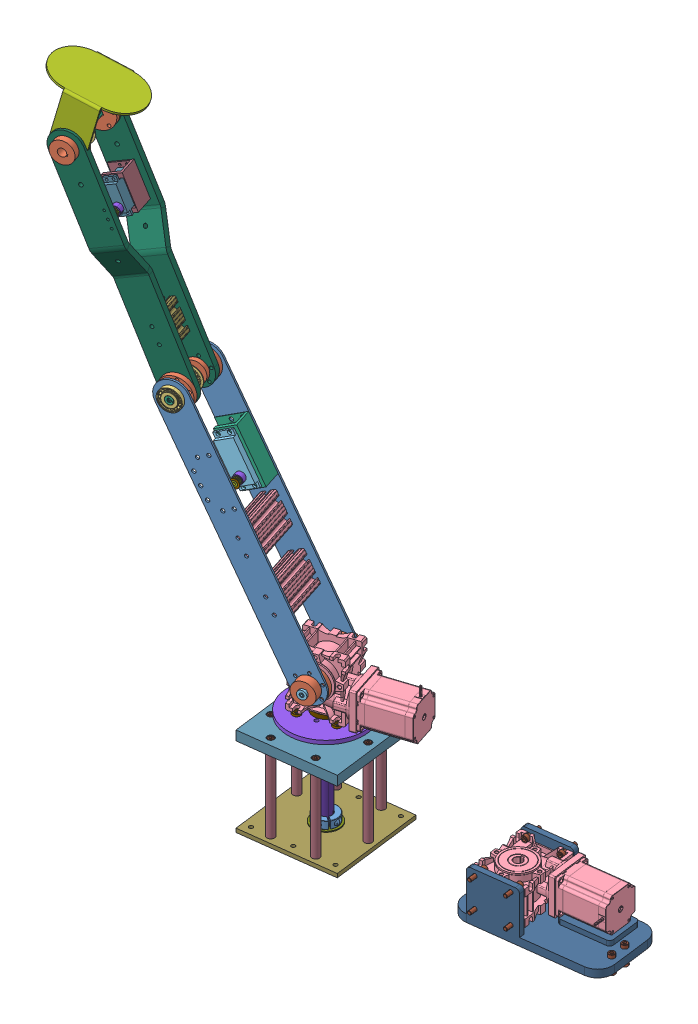
SolidWorks assembly Arm Assembly, configuration Default. Lengths in mm.
Overall size (846.98 1058.59 298.31).
82 component instances, 33 part files, 151 mates.
Components (placement in the parent):
- Link 2-1: Link 2 [Default] at (3.1866 319.7516 325.7135) x (-0.427533 0.893348 0.138367) z (0.307916 0 0.951414) size (457.2 50.8 3.17)
- Keyed hub-1: Keyed hub [Default] at (6.5738 308.3376 409.872) x (0.795226 -0.548979 -0.257367) z (-0.522306 -0.835836 0.169039) size (50.8 25.4 50.8)
- Link 2-2: Link 2 [Default] at (30.6065 319.7516 410.4369) x (-0.427533 0.893348 0.138367) z (0.307916 0 0.951414) size (457.2 50.8 3.17)
- Flanged Bearing-2: Flanged Bearing [Default] at (-163.7305 671.3941 476.7494) x (-0.905825 0.30584 0.293161) z (0.307916 0 0.951414) size (38.1 38.1 12.7)
- Keyed hub-2: Keyed hub [Default] at (-189.4376 671.3941 397.3184) x (-0.113332 -0.99288 0.036679) z (-0.944639 0.11912 0.305723) size (50.8 25.4 50.8)
- Keyed hub-3: Keyed hub [Default] at (-14.9803 308.3376 343.273) x (-0.795226 0.548979 0.257367) z (-0.522306 -0.835836 0.169039) size (50.8 25.4 50.8)
- Keyed hub-4: Keyed hub [Default] at (-166.4679 671.3941 468.2913) x (0.113332 0.99288 -0.036679) z (-0.944639 0.11912 0.305723) size (50.8 25.4 50.8)
- Flanged Bearing-4: Flanged Bearing [Default] at (-192.175 671.3941 388.8603) x (0.893323 0.344073 -0.289115) z (-0.307916 0 -0.951414) size (38.1 38.1 12.7)
- Nema Stepper Motor-2: Nema Stepper Motor [Default] at (66.9639 289.3684 353.54) x (0.951414 0 -0.307916) z (-0.307916 0 -0.951414) size (171.01 100.01 63.01)
- Keyed Drive Shaft-1: Keyed Drive Shaft [Default] at (-40.5477 309.6541 252.9311) x (0.795226 -0.548979 -0.257367) z (0.307916 0 0.951414) size (19.9 19.9 128.01)
- Keyed Shaft-1: Keyed Shaft [Default] at (-196.97 671.3941 374.0443) x (-0.113332 -0.99288 0.036679) z (0.307916 0 0.951414) size (12.7 12.5 104.14)
- Link 4-1: Link 4 [Default] at (-266.4141 1062.3171 464.6146) x (0.307916 0 0.951414) z (0.921727 -0.247856 -0.298308) size (90.37 102.6 133.86)
- Keyed hub-5: Keyed hub [Default] at (-318.7563 993.8869 445.7404) x (0.235814 0.968797 -0.076319) z (-0.921727 0.247856 0.298308) size (50.8 25.4 50.8)
- Keyed hub-6: Keyed hub [Default] at (-297.7724 993.8869 510.5776) x (-0.235814 -0.968797 0.076319) z (-0.921727 0.247856 0.298308) size (50.8 25.4 50.8)
- Joint 2 Motor Plate-1: Joint 2 Motor Plate [Default] at (-4.244 240.9876 376.7854) x (0.894342 0 0.447383) z (-0.447383 0 0.894342) size (127 6.35 127)
- 4 mm M6 spacer-1: 4 mm M6 spacer [94669A162] at (28.8341 249.3376 391.3056) x (-0.888418 0 -0.459036) z (0 -1 0) size (13 13 4)
- 4 mm M6 spacer-2: 4 mm M6 spacer [94669A162] at (-22.5422 249.3376 407.9331) x (0.999963 0 0.008554) z (0 -1 0) size (13 13 4)
- 4 mm M6 spacer-3: 4 mm M6 spacer [94669A162] at (14.0541 249.3376 345.6378) x (1 0 0) z (0 -1 0) size (13 13 4)
- 4 mm M6 spacer-4: 4 mm M6 spacer [94669A162] at (-37.3222 249.3376 362.2652) x (1 0 0) z (0 -1 0) size (13 13 4)
- Motor Mount Joint 1 Assembly-1: Motor Mount Joint 1 Assembly [Default] at (255.7253 -1.2672 148.6448) x (0.992107 0 -0.125391) z (0.125391 0 0.992107) size (228.6 94.85 140.08)
  - Joint 1 Motor Holder Bracket-1: Joint 1 Motor Holder Bracket [Default] at (55.8829 79.1234 191.166) size (228.6 82.55 114.78)
  - Nema Stepper Motor-1: Nema Stepper Motor [Default] at (81.7887 128.4828 180.6968) x (1 0 0) z (0 1 0) size (171.01 100.01 63.01)
  - Flanged Bearing-1: Flanged Bearing [Default] at (6.9829 88.5722 199.666) x (0.99323 0 0.116162) z (0 -1 0) size (38.1 38.1 12.7)
  - socket head cap screw_am-7: socket head cap screw_am [B18.3.1M - 6 x 1.0 x 25 Hex SHCS -- 25NHX] at (-20.0631 152.4828 153.666) x (0 0 -1) z (0.990069 0.140585 0) size (31 10 10)
  - socket head cap screw_am-8: socket head cap screw_am [B18.3.1M - 6 x 1.0 x 25 Hex SHCS -- 25NHX] at (33.9369 152.4828 228.666) x (0 0 1) z (-1 0 0) size (31 10 10)
  - socket head cap screw_am-9: socket head cap screw_am [B18.3.1M - 6 x 1.0 x 25 Hex SHCS -- 25NHX] at (-20.0631 152.4828 228.666) x (0 0 1) z (0.381849 0.924225 0) size (31 10 10)
  - socket head cap screw_am-10: socket head cap screw_am [B18.3.1M - 6 x 1.0 x 25 Hex SHCS -- 25NHX] at (-20.0631 104.4828 153.666) x (0 0 -1) z (0.756248 0.654286 0) size (31 10 10)
  - socket head cap screw_am-11: socket head cap screw_am [B18.3.1M - 6 x 1.0 x 25 Hex SHCS -- 25NHX] at (33.9369 104.4828 150.5881) x (0 0 -1) z (0.923728 0.383049 0) size (31 10 10)
  - socket head cap screw_am-12: socket head cap screw_am [B18.3.1M - 6 x 1.0 x 25 Hex SHCS -- 25NHX] at (-45.7171 97.8234 212.366) x (0 -1 0) z (-0.546944 0 0.837169) size (31 10 10)
  - socket head cap screw_am-19: socket head cap screw_am [B18.3.1M - 6 x 1.0 x 25 Hex SHCS -- 25NHX] at (-45.7171 97.8234 186.966) x (0 -1 0) z (-0.546944 0 0.837169) size (31 10 10)
  - socket head cap screw_am-14: socket head cap screw_am [B18.3.1M - 6 x 1.0 x 25 Hex SHCS -- 25NHX] at (33.9369 152.4828 153.666) x (0 0 -1) z (0.923728 0.383049 0) size (31 10 10)
  - socket head cap screw_am-15: socket head cap screw_am [B18.3.1M - 6 x 1.0 x 25 Hex SHCS -- 25NHX] at (157.4829 97.8234 186.966) x (0 -1 0) z (-0.546944 0 0.837169) size (31 10 10)
  - socket head cap screw_am-16: socket head cap screw_am [B18.3.1M - 6 x 1.0 x 25 Hex SHCS -- 25NHX] at (-20.0631 104.4828 228.666) x (0 0 1) z (-1 0 0) size (31 10 10)
  - socket head cap screw_am-17: socket head cap screw_am [B18.3.1M - 6 x 1.0 x 25 Hex SHCS -- 25NHX] at (33.9369 104.4828 228.666) x (0 0 1) z (-1 0 0) size (31 10 10)
  - socket head cap screw_am-18: socket head cap screw_am [B18.3.1M - 6 x 1.0 x 25 Hex SHCS -- 25NHX] at (157.4829 97.8234 212.366) x (0 -1 0) z (-0.546944 0 0.837169) size (31 10 10)
- Joint 1 bottom plate-1: Joint 1 bottom plate [89155K113] at (-4.244 81.0311 376.7854) x (-0.125391 0 -0.992107) z (0.992107 0 -0.125391) size (152.4 6.35 152.4)
- Base post-1: Base post [8974K269] at (21.393 160.4061 309.54) x (-0.837169 0 -0.546944) z (0 -1 0) size (12.7 12.7 127)
- Base post-2: Base post [8974K269] at (-29.8811 160.4061 444.0308) x (-0.837169 0 -0.546944) z (0 -1 0) size (12.7 12.7 127)
- Base post-3: Base post [8974K269] at (37.3177 160.4061 435.5376) x (0.463623 0 0.886032) z (0 -1 0) size (12.7 12.7 127)
- Base post-4: Base post [8974K269] at (58.7548 160.4061 368.8231) x (-0.837169 0 -0.546944) z (0 -1 0) size (12.7 12.7 127)
- Base post-5: Base post [8974K269] at (-70.4278 160.4061 359.5483) x (-0.837169 0 -0.546944) z (0 -1 0) size (12.7 12.7 127)
- Base post-6: Base post [8974K269] at (-45.8058 160.4061 318.0332) x (-0.837169 0 -0.546944) z (0 -1 0) size (12.7 12.7 127)
- Base post-7: Base post [8974K269] at (-64.0579 160.4061 409.9473) x (-0.837169 0 -0.546944) z (0 -1 0) size (12.7 12.7 127)
- Joint 1 top plate-1: Joint 1 top plate [89155K143] at (-4.244 219.1436 376.7854) x (-0.125391 0 -0.992107) z (0.992107 0 -0.125391) size (152.4 15.88 152.4)
- Tapered-Roller Bearing-1: Tapered-Roller Bearing [5709K77] at (-4.244 223.5886 376.7854) x (1 0 0) z (0 -1 0) size (45.24 45.24 17.1)
- base Ball Bearing 0.75 in-1: base Ball Bearing 0.75 in [6384K367] at (-4.244 79.4436 376.7854) x (1 0 0) z (0 -1 0) size (44.45 44.45 14.27)
- keyed shaft 0.75 in bore 9 in-1: keyed shaft 0.75 in bore 9 in [Default] at (-4.244 140.9751 376.7854) x (0.894342 0 0.447383) z (0 -1 0) size (19.05 18.75 228.6)
- 0.75 in shaft hub-1: 0.75 in shaft hub [Default] at (-4.244 234.6376 376.7854) x (-0.894342 0 -0.447383) z (0 -1 0) size (63.5 63.5 19.49)
- Clamping Two-Piece Shaft Collar 0.75 in-1: Clamping Two-Piece Shaft Collar 0.75 in [6436K16] at (-4.244 92.1436 376.7854) x (0.845517 0 0.533948) z (0 1 0) size (38.06 38.1 12.77)
- T-slot Slider-1: T-slot Slider [5278N52] at (236.9979 67.7205 365.0672) x (-0.837169 0 -0.546944) z (0 1 0) size (10 9.8 4.82)
- T-slot Slider-2: T-slot Slider [5278N52] at (233.8129 65.4156 339.8677) x (-0.837169 0 -0.546944) z (0 1 0) size (10 9.8 4.82)
- T-slot Slider-3: T-slot Slider [5278N52] at (438.5941 68.7454 339.5877) x (-0.838988 0 -0.544149) z (0 1 0) size (10 9.8 4.82)
- T-slot Slider-4: T-slot Slider [5278N52] at (435.4091 66.889 314.3882) x (-0.837169 0 -0.546944) z (0 1 0) size (10 9.8 4.82)
- joint3pulley-1: joint3pulley [6495K752] at (-177.2345 671.3941 435.024) x (0.890627 -0.351711 -0.288243) z (-0.307916 0 -0.951414) size (38.1 38.1 22.23)
- 8020tframeforjoint3-1: 8020tframeforjoint3 [47065T653] at (-63.3123 410.4473 360.7415) x (0.849943 0.449366 -0.275076) z (0.307916 0 0.951414) size (25.4 50.8 85.85)
- 8020tframeforjoint3-2: 8020tframeforjoint3 [47065T653] at (-98.6577 484.3029 372.1807) x (0.849943 0.449366 -0.275076) z (0.307916 0 0.951414) size (25.4 50.8 85.85)
- 80 kg-1: 80 kg [Default] at (-161.425 588.2632 383.1265) x (0.427533 -0.893348 -0.138367) z (-0.849943 -0.449366 0.275076) size (82 48 30)
- servobracket_80kg-1: servobracket_80kg [Default] at (-139.5373 563.5792 375.2419) x (0.427533 -0.893348 -0.138367) z (-0.849943 -0.449366 0.275076) size (87.12 31.24 59.67)
- 3422-0004-0020 assembly.STEP-1: 3422-0004-0020 assembly.STEP [Default] at (-84.0015 538.5018 391.2452) x (0.846926 -0.455616 -0.274099) z (-0.433479 -0.890177 0.140291) size (15 18 15.01)
  - 3422-0004-0020 core.STEP-1: 3422-0004-0020 core.STEP [Default] at (-35.1952 21.4358 6.7264) size (12.22 18 12.22)
  - 3422 series barrel.STEP-1: 3422 series barrel.STEP [Default] at (-35.1952 8.9358 6.7264) x (1 0 0) z (0 1 0) size (15 15.01 9)
  - 3422 series flange.STEP-1: 3422 series flange.STEP [Default] at (-35.1952 24.9358 6.7264) x (1 0 0) z (0 1 0) size (15 15 1)
  - 2806-0005-0005_91390A117.STEP-1: 2806-0005-0005_91390A117.STEP [Default] at (-35.1952 13.4358 11.638) x (-0.412538 -0.91094 0) z (0 0 1) size (5.01 5.01 5.01)
- socket head cap screw_ai-1: socket head cap screw_ai [HX-SHCS 0.25-20x1.5x1-N] at (-29.8811 227.0811 444.0308) x (0 -1 0) z (0 0 1) size (44.45 9.53 9.53)
- socket head cap screw_ai-2: socket head cap screw_ai [HX-SHCS 0.25-20x1.5x1-N] at (-70.4278 227.0811 359.5483) x (0 -1 0) z (0 0 1) size (44.45 9.53 9.53)
- socket head cap screw_ai-3: socket head cap screw_ai [HX-SHCS 0.25-20x1.5x1-N] at (-64.0579 227.0811 409.9473) x (0 -1 0) z (0 0 1) size (44.45 9.53 9.53)
- socket head cap screw_ai-4: socket head cap screw_ai [HX-SHCS 0.25-20x1.5x1-N] at (21.393 227.0811 309.54) x (0 -1 0) z (-0.556107 0 0.831111) size (44.45 9.53 9.53)
- socket head cap screw_ai-5: socket head cap screw_ai [HX-SHCS 0.25-20x1.5x1-N] at (-45.8058 227.0811 318.0332) x (0 -1 0) z (0 0 1) size (44.45 9.53 9.53)
- socket head cap screw_ai-6: socket head cap screw_ai [HX-SHCS 0.25-20x1.5x1-N] at (58.7548 227.0811 368.8231) x (0 -1 0) z (0 0 1) size (44.45 9.53 9.53)
- socket head cap screw_ai-7: socket head cap screw_ai [HX-SHCS 0.25-20x1.5x1-N] at (37.3177 227.0811 435.5376) x (0 -1 0) z (0 0 1) size (44.45 9.53 9.53)
- 8020tframeforjoint4-1: 8020tframeforjoint4 [47065T653] at (-223.9661 741.4538 387.9552) x (-0.874748 -0.393279 0.283104) z (0.307916 0 0.951414) size (25.4 50.8 38.61)
- 25kgservobracket2.step-2: 25kgservobracket2.step [Default] at (-790.2252 -22.9996 653.7215) x (-0.374171 0.919419 0.121097) z (0.307916 0 0.951414) size (55.12 37.85 31.5)
- 25 kg-1: 25 kg [Default] at (-300.4907 914.6985 430.8187) x (0.374171 -0.919419 -0.121097) z (-0.874748 -0.393279 0.283104) size (55 48 20)
- joint3pulley-2: joint3pulley [6495K752] at (-304.6604 993.8869 489.2946) x (-0.682523 -0.696684 0.220892) z (-0.307916 0 -0.951414) size (38.1 38.1 22.23)
- 3422-0004-0020 assembly.STEP-2: 3422-0004-0020 assembly.STEP [Default] at (-264.788 924.7221 452.44) x (0.321984 0.940993 -0.104207) z (0.895273 -0.338427 -0.289747) size (15 18 15.01)
  - 3422-0004-0020 core.STEP-1: 3422-0004-0020 core.STEP [Default] at (-35.1952 21.4358 6.7264) size (12.22 18 12.22)
  - 3422 series barrel.STEP-1: 3422 series barrel.STEP [Default] at (-35.1952 8.9358 6.7264) x (1 0 0) z (0 1 0) size (15 15.01 9)
  - 3422 series flange.STEP-1: 3422 series flange.STEP [Default] at (-35.1952 24.9358 6.7264) x (1 0 0) z (0 1 0) size (15 15 1)
  - 2806-0005-0005_91390A117.STEP-1: 2806-0005-0005_91390A117.STEP [Default] at (-35.1952 13.4358 11.638) x (-0.412538 -0.91094 0) z (0 0 1) size (5.01 5.01 5.01)
- Link 3version2-1: Link 3version2 [Default] at (-149.7725 681.3834 444.0345) x (-0.374171 0.919419 0.121097) z (0.307916 0 0.951414) size (401.56 50.8 32.8)
- Link 3version2-2: Link 3version2 [Default] at (-206.1329 661.4048 421.5752) x (-0.374171 0.919419 0.121097) z (-0.307916 0 -0.951414) size (401.56 50.8 32.8)
- Keyed Shaft-3: Keyed Shaft [Default] at (-329.7058 993.8869 411.9082) x (0.647776 -0.732417 -0.209646) z (0.307916 0 0.951414) size (12.7 12.5 104.14)
Mates (geometry in assembly coordinates):
- Concentric3: concentric aligned: cylinder of Keyed hub-1 through (9.0179 308.3376 417.4238) axis (0.307916 0 0.951414) radius 17.4625; cylinder of Link 2-2 through (9.0179 308.3376 417.4238) axis (0.307916 0 0.951414) radius 17.4625
- Coincident2: coincident anti-aligned: plane of Keyed hub-1 through (9.0179 308.3376 417.4238) normal (0.307916 0 0.951414); plane of Link 2-2 through (9.0179 308.3376 417.4238) normal (-0.307916 0 -0.951414)
- Concentric4: concentric aligned: cylinder of Keyed hub-1 through (25.7829 296.7641 411.998) axis (0.307916 0 0.951414) radius 2.5527; cylinder of Link 2-2 through (26.7605 296.7641 415.0188) axis (0.307916 0 0.951414) radius 2.5527
- Concentric5: concentric anti-aligned: cylinder of Link 2-1 through (-18.402 308.3376 332.7004) axis (0.307916 0 0.951414) radius 17.4625; cylinder of Keyed hub-3 through (-17.4243 308.3376 335.7212) axis (-0.307916 0 -0.951414) radius 17.4625
- Coincident3: coincident anti-aligned: plane of Link 2-1 through (-17.4243 308.3376 335.7212) normal (0.307916 0 0.951414); plane of Keyed hub-3 through (-17.4243 308.3376 335.7212) normal (-0.307916 0 -0.951414)
- Concentric7: concentric anti-aligned: cylinder of Link 2-1 through (-35.3428 298.8641 341.5203) axis (0.307916 0 0.951414) radius 2.5527; cylinder of Keyed hub-3 through (-35.3428 298.8641 341.5203) axis (-0.307916 0 -0.951414) radius 2.5527
- Concentric8: concentric anti-aligned: cylinder of Keyed hub-1 through (6.5738 308.3376 409.872) axis (0.307916 0 0.951414) radius 6.35; cylinder of Keyed hub-3 through (-14.9803 308.3376 343.273) axis (-0.307916 0 -0.951414) radius 6.35
- Coincident5: coincident aligned: plane of Keyed hub-1 through (5.3114 309.2092 410.2806) normal (0.795226 -0.548979 -0.257367); plane of Keyed hub-3 through (-16.2427 309.2092 343.6816) normal (0.795226 -0.548979 -0.257367)
- Concentric9: concentric aligned: cylinder of Link 2-2 through (-164.7316 671.3941 473.6562) axis (0.307916 0 0.951414) radius 17.4625; cylinder of Flanged Bearing-2 through (-161.7752 671.3941 482.7909) axis (0.307916 0 0.951414) radius 17.4625
- Concentric10: concentric anti-aligned: cylinder of Link 2-1 through (-192.1515 671.3941 388.9328) axis (0.307916 0 0.951414) radius 17.4625; cylinder of Flanged Bearing-4 through (-194.1302 671.3941 382.8188) axis (-0.307916 0 -0.951414) radius 17.4625
- Concentric15: concentric anti-aligned: cylinder of Keyed hub-2 through (-189.4376 671.3941 397.3184) axis (0.307916 0 0.951414) radius 6.35; cylinder of Keyed hub-4 through (-166.4679 671.3941 468.2913) axis (-0.307916 0 -0.951414) radius 6.35
- Coincident10: coincident aligned: plane of Keyed hub-2 through (-189.6175 669.8179 397.3766) normal (0.113332 0.99288 -0.036679); plane of Keyed hub-4 through (-166.6478 669.8179 468.3496) normal (0.113332 0.99288 -0.036679)
- Concentric16: concentric aligned: cylinder of Flanged Bearing-2 through (-161.7752 671.3941 482.7909) axis (0.307916 0 0.951414) radius 6.35; cylinder of Keyed hub-2 through (-189.4376 671.3941 397.3184) axis (0.307916 0 0.951414) radius 6.35
- Concentric21: concentric anti-aligned: cylinder of Keyed hub-1 through (6.5738 308.3376 409.872) axis (0.307916 0 0.951414) radius 6.35; cylinder of Keyed Drive Shaft-1 through (15.5034 308.3376 437.463) axis (-0.307916 0 -0.951414) radius 7
- Parallel1: parallel anti-aligned: plane of Keyed hub-1 through (5.3114 309.2092 410.2806) normal (0.795226 -0.548979 -0.257367); plane of Keyed Drive Shaft-1 through (-3.4231 314.14 376.32) normal (-0.795226 0.548979 0.257367)
- Coincident18: coincident anti-aligned: plane of Keyed hub-3 through (-14.9803 308.3376 343.273) normal (0.307916 0 0.951414); plane of Keyed Drive Shaft-1 through (-12.4386 314.5909 342.4504) normal (-0.307916 0 -0.951414)
- Coincident19: coincident anti-aligned: plane of Keyed hub-1 through (6.5738 308.3376 409.872) normal (-0.307916 0 -0.951414); plane of Keyed Drive Shaft-1 through (9.1155 314.5909 409.0494) normal (0.307916 0 0.951414)
- Concentric22: concentric anti-aligned: cylinder of Keyed hub-2 through (-189.4376 671.3941 397.3184) axis (0.307916 0 0.951414) radius 6.35; cylinder of Keyed Shaft-1 through (-161.7752 671.3941 482.7909) axis (-0.307916 0 -0.951414) radius 6.35
- Coincident20: coincident aligned: plane of Keyed hub-2 through (-189.6175 669.8179 397.3766) normal (0.113332 0.99288 -0.036679); plane of Keyed Shaft-1 through (-157.4683 669.2521 481.397) normal (0.113332 0.99288 -0.036679)
- Coincident22: coincident anti-aligned: plane of Link 2-1 through (-17.4243 308.3376 335.7212) normal (0.307916 0 0.951414); plane of Flanged Bearing-4 through (-185.4574 654.9978 390.1035) normal (-0.307916 0 -0.951414)
- Distance1: distance = 2.54 mm anti-aligned: plane of Flanged Bearing-4 through (-186.4531 660.5904 393.6827) normal (0.307916 0 0.951414); plane of Keyed hub-2 through (-189.4376 671.3941 397.3184) normal (-0.307916 0 -0.951414)
- Coincident24: coincident anti-aligned: plane of Link 2-2 through (9.0179 308.3376 417.4238) normal (-0.307916 0 -0.951414); plane of Flanged Bearing-2 through (-169.8128 654.7683 475.3007) normal (0.307916 0 0.951414)
- Distance2: distance = 2.54 mm anti-aligned: plane of Keyed hub-4 through (-166.4679 671.3941 468.2913) normal (0.307916 0 0.951414); plane of Flanged Bearing-2 through (-169.0338 660.4392 471.7915) normal (-0.307916 0 -0.951414)
- Coincident26: coincident aligned: plane of Flanged Bearing-2 through (-163.623 665.3484 483.3889) normal (0.307916 0 0.951414); plane of Keyed Shaft-1 through (-161.7752 671.3941 482.7909) normal (0.307916 0 0.951414)
- Concentric23: concentric anti-aligned: cylinder of Link 4-1 through (-294.3507 993.8869 521.1502) axis (-0.307916 0 -0.951414) radius 17.4625; cylinder of Keyed hub-6 through (-295.3283 993.8869 518.1294) axis (0.307916 0 0.951414) radius 17.4625
- Concentric24: concentric anti-aligned: cylinder of Link 4-1 through (-280.9856 979.1495 513.4875) axis (-0.307916 0 -0.951414) radius 2.5527; cylinder of Keyed hub-6 through (-280.9856 979.1495 513.4875) axis (0.307916 0 0.951414) radius 2.5527
- Coincident27: coincident anti-aligned: plane of Link 4-1 through (-243.8064 1102.0514 501.4549) normal (-0.307916 0 -0.951414); plane of Keyed hub-6 through (-295.3283 993.8869 518.1294) normal (0.307916 0 0.951414)
- Concentric25: concentric anti-aligned: cylinder of Link 4-1 through (-322.178 993.8869 435.1679) axis (0.307916 0 0.951414) radius 17.4625; cylinder of Keyed hub-5 through (-321.2004 993.8869 438.1886) axis (-0.307916 0 -0.951414) radius 17.4625
- Concentric26: concentric anti-aligned: cylinder of Link 4-1 through (-306.8576 979.1495 433.5467) axis (0.307916 0 0.951414) radius 2.5527; cylinder of Keyed hub-5 through (-306.8576 979.1495 433.5467) axis (-0.307916 0 -0.951414) radius 2.5527
- Coincident34: coincident anti-aligned: plane of Link 4-1 through (-269.6785 1102.0514 421.514) normal (0.307916 0 0.951414); plane of Keyed hub-5 through (-321.2004 993.8869 438.1886) normal (-0.307916 0 -0.951414)
- Coincident38: coincident anti-aligned: plane of Top base plate-1 through (74.0847 244.0001 261.2257) normal (0 -1 0); plane of arm base spacer small part-1 through (130.8381 244.0001 364.6329) normal (0 1 0)
- Coincident40: coincident anti-aligned: plane of Top base plate-1 through (74.0847 244.0001 261.2257) normal (0 -1 0); plane of arm base spacer large part-1 through (32.1724 244.0001 346.1862) normal (0 1 0)
- Coincident45: coincident anti-aligned: plane of Bearing other part-1 through (32.1724 247.1751 346.1862) normal (0 -1 0); plane of Top base plate-1 through (74.0847 247.1751 261.2257) normal (0 1 0)
- Concentric32: concentric aligned: cylinder of Bearing other part-1 through (32.1724 257.1751 346.1862) axis (0 -1 0) radius 70; circle of arm base spacer large part-1
- Coincident57: coincident aligned: plane of Top base plate-1 through (-6.0476 247.1751 446.2586) normal (0.059501 0 0.998228); plane of arm base spacer large part-1 through (84.7912 244.0001 440.844) normal (0.059501 0 0.998228)
- Coincident58: coincident aligned: plane of Top base plate-1 through (-75.7951 247.1751 376.9496) normal (-0.998228 0 0.059501); plane of arm base spacer large part-1 through (-75.8042 244.0001 376.7975) normal (-0.998228 0 0.059501)
- Concentric37: concentric aligned: cylinder of Top base plate-1 through (130.8381 247.1751 364.6329) axis (0 -1 0) radius 15; cylinder of arm base spacer small part-1 through (130.8381 244.0001 364.6329) axis (0 -1 0) radius 15
- Coincident59: coincident aligned: plane of Top base plate-1 through (145.8116 247.1751 363.7404) normal (0.998228 0 -0.059501); plane of arm base spacer small part-1 through (145.8116 244.0001 363.7404) normal (0.998228 0 -0.059501)
- Parallel2: parallel aligned: plane of Nema Stepper Motor-3 through (350.3499 203.0272 320.7095) normal (0 1 0); plane of Top base plate-1 through (74.0847 247.1751 261.2257) normal (0 1 0)
- Parallel3: parallel anti-aligned: plane of Nema Stepper Motor-3 through (312.2058 175.0272 353.0364) normal (-0.998228 0 0.059501); plane of arm base spacer small part-1 through (145.8116 244.0001 363.7404) normal (0.998228 0 -0.059501)
- Coincident61: coincident anti-aligned: plane of Nema Stepper Motor-2 through (42.4708 251.3376 390.8968) normal (0 -1 0); plane of 4 mm M6 spacer-1 through (28.8341 251.3376 391.3056) normal (0 1 0)
- Concentric43: concentric aligned: cylinder of Keyed hub-1 through (9.0179 308.3376 417.4238) axis (0.307916 0 0.951414) radius 17.4625; cylinder of Nema Stepper Motor-2 through (-32.7548 308.3376 288.3523) axis (0.307916 0 0.951414) radius 7
- Coincident65: coincident anti-aligned: plane of Nema Stepper Motor-2 through (5.4919 308.3376 406.5434) normal (0.307916 0 0.951414); plane of Keyed Drive Shaft-1 through (5.4961 308.3376 406.542) normal (-0.307916 0 -0.951414)
- Concentric44: concentric aligned: cylinder of Joint 1 bottom plate-1 through (58.7548 83.9521 368.8231) axis (0 1 0) radius 1.905; cylinder of Base post-4 through (58.7548 84.2061 368.8231) axis (0 1 0) radius 6.35
- Concentric45: concentric aligned: cylinder of Joint 1 bottom plate-1 through (37.3177 83.9521 435.5376) axis (0 1 0) radius 1.905; cylinder of Base post-3 through (37.3177 84.2061 435.5376) axis (0 1 0) radius 6.35
- Concentric46: concentric aligned: cylinder of Joint 1 bottom plate-1 through (-29.8811 83.9521 444.0308) axis (0 1 0) radius 1.905; cylinder of Base post-2 through (-29.8811 84.2061 444.0308) axis (0 1 0) radius 6.35
- Concentric47: concentric aligned: cylinder of Joint 1 bottom plate-1 through (21.393 83.9521 309.54) axis (0 1 0) radius 1.905; cylinder of Base post-1 through (21.393 84.2061 309.54) axis (0 1 0) radius 6.35
- Concentric48: concentric aligned: cylinder of Joint 1 bottom plate-1 through (-45.8058 83.9521 318.0332) axis (0 1 0) radius 1.905; cylinder of Base post-6 through (-45.8058 84.2061 318.0332) axis (0 1 0) radius 6.35
- Concentric49: concentric aligned: cylinder of Joint 1 bottom plate-1 through (-64.0579 83.9521 409.9473) axis (0 1 0) radius 1.905; cylinder of Base post-7 through (-64.0579 84.2061 409.9473) axis (0 1 0) radius 6.35
- Concentric50: concentric aligned: cylinder of Joint 1 bottom plate-1 through (-70.4278 83.9521 359.5483) axis (0 1 0) radius 1.905; cylinder of Base post-5 through (-70.4278 84.2061 359.5483) axis (0 1 0) radius 6.35
- Coincident66: coincident anti-aligned: plane of Joint 1 bottom plate-1 through (80.9094 84.2061 442.8292) normal (0 1 0); plane of Base post-4 through (58.7548 84.2061 368.8231) normal (0 -1 0)
- Coincident67: coincident anti-aligned: plane of Joint 1 bottom plate-1 through (80.9094 84.2061 442.8292) normal (0 1 0); plane of Base post-3 through (37.3177 84.2061 435.5376) normal (0 -1 0)
- Coincident68: coincident anti-aligned: plane of Joint 1 bottom plate-1 through (80.9094 84.2061 442.8292) normal (0 1 0); plane of Base post-2 through (-29.8811 84.2061 444.0308) normal (0 -1 0)
- Coincident69: coincident anti-aligned: plane of Joint 1 bottom plate-1 through (80.9094 84.2061 442.8292) normal (0 1 0); plane of Base post-7 through (-64.0579 84.2061 409.9473) normal (0 -1 0)
- Coincident70: coincident anti-aligned: plane of Joint 1 bottom plate-1 through (80.9094 84.2061 442.8292) normal (0 1 0); plane of Base post-1 through (21.393 84.2061 309.54) normal (0 -1 0)
- Coincident71: coincident anti-aligned: plane of Joint 1 bottom plate-1 through (80.9094 84.2061 442.8292) normal (0 1 0); plane of Base post-6 through (-45.8058 84.2061 318.0332) normal (0 -1 0)
- Coincident72: coincident anti-aligned: plane of Joint 1 bottom plate-1 through (80.9094 84.2061 442.8292) normal (0 1 0); plane of Base post-5 through (-70.4278 84.2061 359.5483) normal (0 -1 0)
- Coincident75: coincident anti-aligned: plane of Base post-3 through (37.3177 211.2061 435.5376) normal (0 1 0); plane of Joint 1 top plate-1 through (61.7997 211.2061 291.632) normal (0 -1 0)
- Parallel5: parallel aligned: plane of Motor Mount Joint 1 Assembly-1/Joint 1 Motor Holder Bracket-1 through (228.936 90.5561 402.5641) normal (0.125391 0 0.992107); plane of Joint 1 bottom plate-1 through (80.9094 77.8561 442.8292) normal (0.125391 0 0.992107)
- Coincident79: coincident anti-aligned: plane of Joint 1 top plate-1 through (-4.244 217.5561 376.7854) normal (0 1 0); plane of Tapered-Roller Bearing-1 through (-4.244 217.5561 399.4073) normal (0 -1 0)
- Concentric51: concentric anti-aligned: cylinder of Joint 1 top plate-1 through (-4.244 217.5561 376.7854) axis (0 1 0) radius 22.6219; cylinder of Tapered-Roller Bearing-1 through (-4.244 223.5886 376.7854) axis (0 -1 0) radius 22.6219
- Coincident80: coincident anti-aligned: plane of Nema Stepper Motor-2 through (42.4708 251.3376 390.8968) normal (0 -1 0); plane of 4 mm M6 spacer-2 through (-22.5422 251.3376 407.9331) normal (0 1 0)
- Coincident81: coincident anti-aligned: plane of Nema Stepper Motor-2 through (42.4708 251.3376 390.8968) normal (0 -1 0); plane of 4 mm M6 spacer-4 through (-37.3222 251.3376 362.2652) normal (0 1 0)
- Concentric52: concentric anti-aligned: cylinder of Joint 1 bottom plate-1 through (-4.244 77.8561 376.7854) axis (0 1 0) radius 20.6375; cylinder of base Ball Bearing 0.75 in-1 through (-4.244 73.0936 376.7854) axis (0 -1 0) radius 20.6375
- Coincident82: coincident anti-aligned: plane of Joint 1 bottom plate-1 through (80.9094 84.2061 442.8292) normal (0 1 0); plane of base Ball Bearing 0.75 in-1 through (-4.244 84.2061 395.7927) normal (0 -1 0)
- Concentric53: concentric anti-aligned: cylinder of base Ball Bearing 0.75 in-1 through (-4.244 73.0936 376.7854) axis (0 -1 0) radius 9.525; cylinder of keyed shaft 0.75 in bore-1 through (-4.244 -126.3486 376.7854) axis (0 1 0) radius 9.525
- Concentric54: concentric anti-aligned: cylinder of base Ball Bearing 0.75 in-1 through (-4.244 73.0936 376.7854) axis (0 -1 0) radius 9.525; cylinder of keyed shaft 0.75 in bore 9 in-1 through (-4.244 26.6751 376.7854) axis (0 1 0) radius 9.525
- Coincident83: coincident aligned: plane of Motor Mount Joint 1 Assembly-1/Joint 1 Motor Holder Bracket-1 through (335.1377 77.8561 331.2948) normal (0 -1 0); plane of Joint 1 bottom plate-1 through (61.7997 77.8561 291.632) normal (0 -1 0)
- Concentric55: concentric aligned: cylinder of Joint 2 Motor Plate-1 through (-4.244 240.9876 376.7854) axis (0 1 0) radius 20.6375; circle of 0.75 in shaft hub-1
- Concentric56: concentric anti-aligned: cylinder of Joint 2 Motor Plate-1 through (-12.2717 240.9876 352.6873) axis (0 1 0) radius 3.175; circle of 0.75 in shaft hub-1
- Concentric57: concentric aligned: cylinder of keyed shaft 0.75 in bore 9 in-1 through (-4.244 26.6751 376.7854) axis (0 1 0) radius 9.525; cylinder of 0.75 in shaft hub-1 through (-4.244 233.0501 376.7854) axis (0 1 0) radius 9.525
- Parallel6: parallel aligned: plane of keyed shaft 0.75 in bore 9 in-1 through (-9.5725 26.6751 382.1005) normal (0.894342 0 0.447383); plane of 0.75 in shaft hub-1 through (-11.7003 234.6376 386.3684) normal (0.894342 0 0.447383)
- Coincident90: coincident anti-aligned: plane of Joint 2 Motor Plate-1 through (-4.244 240.9876 376.7854) normal (0 -1 0); plane of 0.75 in shaft hub-1 through (-4.244 240.9876 376.7854) normal (0 1 0)
- Concentric60: concentric anti-aligned: cylinder of keyed shaft 0.75 in bore 9 in-1 through (-4.244 26.6751 376.7854) axis (0 1 0) radius 9.525; cylinder of Clamping Two-Piece Shaft Collar 0.75 in-1 through (-4.244 98.4936 376.7854) axis (0 -1 0) radius 9.525
- Distance9: distance = 1.5875 mm aligned: plane of keyed shaft 0.75 in bore 9 in-1 through (-4.244 255.2751 376.7854) normal (0 1 0); plane of 0.75 in shaft hub-1 through (-4.244 253.6876 376.7854) normal (0 1 0)
- Coincident95: coincident anti-aligned: plane of Nema Stepper Motor-2 through (42.4708 251.3376 390.8968) normal (0 -1 0); plane of 4 mm M6 spacer-3 through (14.0541 251.3376 345.6378) normal (0 1 0)
- Coincident96: coincident anti-aligned: plane of Joint 2 Motor Plate-1 through (-4.244 247.3376 376.7854) normal (0 1 0); plane of 4 mm M6 spacer-3 through (14.0541 247.3376 345.6378) normal (0 -1 0)
- Concentric62: concentric anti-aligned: cylinder of Joint 2 Motor Plate-1 through (28.8341 240.9876 391.3056) axis (0 1 0) radius 3.25; cylinder of 4 mm M6 spacer-1 through (28.8341 251.3376 391.3056) axis (0 -1 0) radius 3.15
- Concentric63: concentric anti-aligned: cylinder of Joint 2 Motor Plate-1 through (-22.5422 240.9876 407.9331) axis (0 1 0) radius 3.25; cylinder of 4 mm M6 spacer-2 through (-22.5422 251.3376 407.9331) axis (0 -1 0) radius 3.15
- Tangent1: tangent anti-aligned: plane of Nema Stepper Motor-2 through (25.1628 274.039 390.192) normal (0.951414 0 -0.307916); cylinder of 4 mm M6 spacer-1 through (28.8341 251.3376 391.3056) axis (0 -1 0) radius 3.15
- Tangent2: tangent anti-aligned: plane of Nema Stepper Motor-2 through (-26.2135 274.039 406.8194) normal (0.951414 0 -0.307916); cylinder of 4 mm M6 spacer-2 through (-22.5422 251.3376 407.9331) axis (0 -1 0) radius 3.15
- Tangent3: tangent anti-aligned: plane of Nema Stepper Motor-2 through (11.6145 274.039 348.3298) normal (0.951414 0 -0.307916); cylinder of 4 mm M6 spacer-3 through (14.0541 251.3376 345.6378) axis (0 -1 0) radius 3.15
- Concentric67: concentric anti-aligned: cylinder of Joint 2 Motor Plate-1 through (-37.3222 240.9876 362.2652) axis (0 1 0) radius 3.25; cylinder of 4 mm M6 spacer-4 through (-37.3222 251.3376 362.2652) axis (0 -1 0) radius 3.15
- Tangent5: tangent anti-aligned: plane of Nema Stepper Motor-2 through (-39.7618 274.039 364.9572) normal (0.951414 0 -0.307916); cylinder of 4 mm M6 spacer-4 through (-37.3222 251.3376 362.2652) axis (0 -1 0) radius 3.15
- Concentric68: concentric anti-aligned: cylinder of Joint 2 Motor Plate-1 through (14.0541 240.9876 345.6378) axis (0 1 0) radius 3.25; cylinder of 4 mm M6 spacer-3 through (14.0541 251.3376 345.6378) axis (0 -1 0) radius 3.15
- Distance11: distance = 3.81 mm: point of 4 mm M6 spacer-1; plane of Nema Stepper Motor-2 through (4.4142 308.3376 403.2134) normal (0.307916 0 0.951414)
- Concentric69: concentric aligned: cylinder of Motor Mount Joint 1 Assembly-1/socket head cap screw_am-18 through (438.5941 128.3061 339.5877) axis (0 1 0) radius 3; circle of T-slot Slider-3
- Concentric70: concentric aligned: cylinder of Motor Mount Joint 1 Assembly-1/socket head cap screw_am-15 through (435.4091 128.3061 314.3882) axis (0 1 0) radius 3; circle of T-slot Slider-4
- Concentric71: concentric aligned: cylinder of Motor Mount Joint 1 Assembly-1/socket head cap screw_am-12 through (236.9979 128.3061 365.0672) axis (0 1 0) radius 3; circle of T-slot Slider-1
- Concentric72: concentric aligned: cylinder of Motor Mount Joint 1 Assembly-1/socket head cap screw_am-19 through (233.8129 128.3061 339.8677) axis (0 1 0) radius 3; circle of T-slot Slider-2
- Concentric74: concentric anti-aligned: cylinder of Link 2-2 through (-45.2788 421.7928 434.9964) axis (0.307916 0 0.951414) radius 2.794; cylinder of 8020tframeforjoint3-1 through (-45.2788 421.7928 434.9964) axis (-0.307916 0 -0.951414) radius 2.6035
- Concentric75: concentric anti-aligned: cylinder of Link 2-2 through (-34.4195 399.1018 431.4819) axis (0.307916 0 0.951414) radius 2.794; cylinder of 8020tframeforjoint3-1 through (-34.4195 399.1018 431.4819) axis (-0.307916 0 -0.951414) radius 2.6035
- Coincident98: coincident anti-aligned: plane of Link 2-2 through (9.0179 308.3376 417.4238) normal (-0.307916 0 -0.951414); plane of 8020tframeforjoint3-1 through (-25.8297 390.4783 428.7019) normal (0.307916 0 0.951414)
- Concentric76: concentric anti-aligned: cylinder of Link 2-2 through (-80.6242 495.6485 446.4356) axis (0.307916 0 0.951414) radius 2.794; cylinder of 8020tframeforjoint3-2 through (-80.6242 495.6485 446.4356) axis (-0.307916 0 -0.951414) radius 2.6035
- Concentric77: concentric anti-aligned: cylinder of Link 2-2 through (-69.7649 472.9574 442.9211) axis (0.307916 0 0.951414) radius 2.794; cylinder of 8020tframeforjoint3-2 through (-69.7649 472.9574 442.9211) axis (-0.307916 0 -0.951414) radius 2.6035
- Coincident99: coincident anti-aligned: plane of Link 2-2 through (9.0179 308.3376 417.4238) normal (-0.307916 0 -0.951414); plane of 8020tframeforjoint3-2 through (-61.1752 464.3339 440.1411) normal (0.307916 0 0.951414)
- Coincident100: coincident anti-aligned: plane of 80 kg-1 through (-161.425 588.2632 383.1265) normal (-0.307916 0 -0.951414); plane of servobracket_80kg-1 through (-139.3027 563.5792 375.9668) normal (0.307916 0 0.951414)
- Concentric78: concentric aligned: cylinder of 80 kg-1 through (-111.524 536.2889 366.9765) axis (0.307916 0 0.951414) radius 3; cylinder of servobracket_80kg-1 through (-111.7586 536.2889 366.2516) axis (0.307916 0 0.951414) radius 3
- Concentric79: concentric aligned: cylinder of 80 kg-1 through (-158.038 595.6508 382.0303) axis (0.307916 0 0.951414) radius 3; cylinder of servobracket_80kg-1 through (-158.2727 595.6508 381.3054) axis (0.307916 0 0.951414) radius 3
- Concentric80: concentric aligned: cylinder of 80 kg-1 through (-111.6642 548.5496 417.4731) axis (-0.307916 0 -0.951414) radius 2; cylinder of 3422-0004-0020 assembly.STEP-1/3422-0004-0020 core.STEP-1 through (-104.6659 548.5496 439.0968) axis (-0.307916 0 -0.951414) radius 2
- Coincident101: coincident anti-aligned: plane of 80 kg-1 through (-148.9544 588.2632 421.6588) normal (0.307916 0 0.951414); plane of 3422-0004-0020 assembly.STEP-1/3422 series barrel.STEP-1 through (-113.9735 548.5496 410.3375) normal (-0.307916 0 -0.951414)
- Coincident102: coincident anti-aligned: plane of Link 2-1 through (-17.4243 308.3376 335.7212) normal (0.307916 0 0.951414); plane of servobracket_80kg-1 through (-139.5373 563.5792 375.2419) normal (-0.307916 0 -0.951414)
- Concentric83: concentric aligned: cylinder of Link 2-1 through (-155.2264 555.8013 376.9823) axis (0.307916 0 0.951414) radius 3.048; circle of servobracket_80kg-1
- Concentric85: concentric aligned: cylinder of Link 2-1 through (-146.5389 537.6485 374.1707) axis (0.307916 0 0.951414) radius 3.048; cylinder of servobracket_80kg-1 through (-145.5613 537.6485 377.1915) axis (0.307916 0 0.951414) radius 3
- Concentric86: concentric aligned: cylinder of Link 2-1 through (-163.9139 573.9541 379.7939) axis (0.307916 0 0.951414) radius 3.048; cylinder of servobracket_80kg-1 through (-162.9362 573.9541 382.8147) axis (0.307916 0 0.951414) radius 3
- Concentric91: concentric aligned: cylinder of Keyed Shaft-1 through (-161.7752 671.3941 482.7909) axis (-0.307916 0 -0.951414) radius 6.35; cylinder of joint3pulley-1 through (-180.6562 671.3941 424.4514) axis (-0.307916 0 -0.951414) radius 6.35
- Parallel9: parallel aligned: cylinder of joint3pulley-1 through (-180.6562 671.3941 424.4514) axis (-0.307916 0 -0.951414) radius 19.05; cylinder of 3422-0004-0020 assembly.STEP-1/3422 series flange.STEP-1 through (-108.739 548.5496 426.5116) axis (-0.307916 0 -0.951414) radius 7.5
- Distance12: distance = 1.5875 mm anti-aligned: plane of 0.75 in shaft hub-1 through (-4.244 234.6376 376.7854) normal (0 -1 0); plane of Tapered-Roller Bearing-1 through (-4.244 233.0501 386.3104) normal (0 1 0)
- Coincident104: coincident anti-aligned: plane of base Ball Bearing 0.75 in-1 through (-4.244 85.7936 376.7854) normal (0 1 0); plane of Clamping Two-Piece Shaft Collar 0.75 in-1 through (-4.244 85.7936 376.7854) normal (0 -1 0)
- Concentric92: concentric aligned: cylinder of Base post-2 through (-29.8811 211.2061 444.0308) axis (0 1 0) radius 3.175; cylinder of Joint 1 top plate-1 through (-29.8811 227.0811 444.0308) axis (0 1 0) radius 5.5563
- Concentric93: concentric aligned: cylinder of Base post-1 through (21.393 211.2061 309.54) axis (0 1 0) radius 3.175; cylinder of Joint 1 top plate-1 through (21.393 227.0811 309.54) axis (0 1 0) radius 5.5563
- Concentric94: concentric aligned: cylinder of Joint 1 top plate-1 through (21.393 227.0811 309.54) axis (0 1 0) radius 3.3782; cylinder of socket head cap screw_ai-4 through (21.393 258.8311 309.54) axis (0 1 0) radius 3.175
- Coincident105: coincident anti-aligned: plane of Joint 1 top plate-1 through (20.9694 220.7311 306.1885) normal (0 1 0); plane of socket head cap screw_ai-4 through (25.3511 220.7311 312.1885) normal (0 -1 0)
- Coincident106: coincident anti-aligned: plane of Joint 1 top plate-1 through (-46.2294 220.7311 314.6817) normal (0 1 0); plane of socket head cap screw_ai-5 through (-41.0433 220.7311 318.0332) normal (0 -1 0)
- Concentric96: concentric aligned: cylinder of Base post-6 through (-45.8058 84.2061 318.0332) axis (0 1 0) radius 6.35; cylinder of socket head cap screw_ai-5 through (-45.8058 258.8311 318.0332) axis (0 1 0) radius 3.175
- Coincident107: coincident anti-aligned: plane of Joint 1 top plate-1 through (36.8941 220.7311 432.1861) normal (0 1 0); plane of socket head cap screw_ai-7 through (42.0802 220.7311 435.5376) normal (0 -1 0)
- Coincident108: coincident anti-aligned: plane of Joint 1 top plate-1 through (-30.3047 220.7311 440.6793) normal (0 1 0); plane of socket head cap screw_ai-1 through (-25.1186 220.7311 444.0308) normal (0 -1 0)
- Coincident109: coincident anti-aligned: plane of Joint 1 top plate-1 through (-64.4815 220.7311 406.5958) normal (0 1 0); plane of socket head cap screw_ai-3 through (-59.2954 220.7311 409.9473) normal (0 -1 0)
- Coincident110: coincident anti-aligned: plane of Joint 1 top plate-1 through (-70.8514 220.7311 356.1967) normal (0 1 0); plane of socket head cap screw_ai-2 through (-65.6653 220.7311 359.5483) normal (0 -1 0)
- Concentric97: concentric aligned: cylinder of Base post-5 through (-70.4278 84.2061 359.5483) axis (0 1 0) radius 6.35; cylinder of socket head cap screw_ai-2 through (-70.4278 258.8311 359.5483) axis (0 1 0) radius 3.175
- Concentric98: concentric aligned: cylinder of Base post-7 through (-64.0579 84.2061 409.9473) axis (0 1 0) radius 6.35; cylinder of socket head cap screw_ai-3 through (-64.0579 258.8311 409.9473) axis (0 1 0) radius 3.175
- Coincident111: coincident anti-aligned: plane of Joint 1 top plate-1 through (58.3312 220.7311 365.4715) normal (0 1 0); plane of socket head cap screw_ai-6 through (63.5173 220.7311 368.8231) normal (0 -1 0)
- Concentric99: concentric aligned: cylinder of Joint 1 top plate-1 through (58.7548 227.0811 368.8231) axis (0 1 0) radius 3.3782; cylinder of socket head cap screw_ai-6 through (58.7548 258.8311 368.8231) axis (0 1 0) radius 3.175
- Concentric100: concentric aligned: cylinder of Joint 1 top plate-1 through (37.3177 227.0811 435.5376) axis (0 1 0) radius 5.5563; cylinder of socket head cap screw_ai-7 through (37.3177 258.8311 435.5376) axis (0 1 0) radius 3.175
- Concentric101: concentric aligned: cylinder of Joint 1 top plate-1 through (-29.8811 227.0811 444.0308) axis (0 1 0) radius 5.5563; cylinder of socket head cap screw_ai-1 through (-29.8811 258.8311 444.0308) axis (0 1 0) radius 3.175
- Concentric109: concentric aligned: cylinder of 25kgservobracket2.step-2 through (-298.3022 920.1128 427.4407) axis (0.307916 0 0.951414) radius 1.875; cylinder of 25 kg-1 through (-297.5201 920.1128 429.8573) axis (0.307916 0 0.951414) radius 1.875
- Coincident115: coincident aligned: cylinder of 25kgservobracket2.step-2 through (-280.529 876.4404 421.6886) axis (0.307916 0 0.951414) radius 1.875; circle of 25 kg-1
- Coincident116: coincident anti-aligned: plane of 25kgservobracket2.step-2 through (-809.093 -22.9996 595.4229) normal (0.307916 0 0.951414); plane of 25 kg-1 through (-300.4907 914.6985 430.8187) normal (-0.307916 0 -0.951414)
- Concentric110: concentric anti-aligned: cylinder of Keyed hub-4 through (-168.912 671.3941 460.7395) axis (-0.307916 0 -0.951414) radius 17.4625; cylinder of Link 3version2-1 through (-171.9911 671.3941 451.2254) axis (0.307916 0 0.951414) radius 17.4625
- Concentric111: concentric anti-aligned: cylinder of Keyed hub-4 through (-187.3534 663.103 466.7079) axis (-0.307916 0 -0.951414) radius 2.5527; cylinder of Link 3version2-1 through (-190.4325 663.103 457.1937) axis (0.307916 0 0.951414) radius 2.5527
- Coincident117: coincident anti-aligned: plane of Keyed hub-4 through (-168.912 671.3941 460.7395) normal (-0.307916 0 -0.951414); plane of Link 3version2-1 through (-168.912 671.3941 460.7395) normal (0.307916 0 0.951414)
- Concentric112: concentric aligned: cylinder of Keyed Shaft-1 through (-161.7752 671.3941 482.7909) axis (-0.307916 0 -0.951414) radius 6.35; cylinder of Link 3version2-2 through (-183.9143 671.3941 414.3843) axis (-0.307916 0 -0.951414) radius 17.4625
- Coincident118: coincident anti-aligned: plane of Keyed hub-2 through (-186.9935 671.3941 404.8702) normal (0.307916 0 0.951414); plane of Link 3version2-2 through (-186.9935 671.3941 404.8702) normal (-0.307916 0 -0.951414)
- Concentric113: concentric anti-aligned: cylinder of Keyed hub-2 through (-203.0457 684.0349 410.0653) axis (0.307916 0 0.951414) radius 2.5527; cylinder of Link 3version2-2 through (-199.9665 684.0349 419.5795) axis (-0.307916 0 -0.951414) radius 2.5527
- Coincident121: coincident anti-aligned: plane of 8020tframeforjoint4-1 through (-213.321 762.2956 464.6014) normal (0.307916 0 0.951414); plane of Link 3version2-1 through (-171.9911 671.3941 451.2254) normal (-0.307916 0 -0.951414)
- Concentric114: concentric anti-aligned: cylinder of 8020tframeforjoint4-1 through (-205.2549 753.1305 461.9909) axis (-0.307916 0 -0.951414) radius 2.6035; cylinder of Link 3version2-1 through (-205.2549 753.1305 461.9909) axis (0.307916 0 0.951414) radius 2.794
- Concentric115: concentric anti-aligned: cylinder of 8020tframeforjoint4-1 through (-195.751 729.7772 458.915) axis (-0.307916 0 -0.951414) radius 2.6035; cylinder of Link 3version2-1 through (-195.751 729.7772 458.915) axis (0.307916 0 0.951414) radius 2.794
- Concentric118: concentric anti-aligned: cylinder of 25kgservobracket2.step-2 through (-295.22 882.4357 426.4432) axis (0.307916 0 0.951414) radius 1.905; cylinder of Link 3version2-2 through (-295.22 882.4357 426.4432) axis (-0.307916 0 -0.951414) radius 1.905
- Concentric119: concentric anti-aligned: cylinder of 25kgservobracket2.step-2 through (-299.972 894.1123 427.9811) axis (0.307916 0 0.951414) radius 1.905; cylinder of Link 3version2-2 through (-299.972 894.1123 427.9811) axis (-0.307916 0 -0.951414) radius 1.905
- Concentric120: concentric anti-aligned: cylinder of 25kgservobracket2.step-2 through (-304.724 905.789 429.519) axis (0.307916 0 0.951414) radius 1.905; cylinder of Link 3version2-2 through (-304.724 905.789 429.519) axis (-0.307916 0 -0.951414) radius 1.905
- Coincident128: coincident anti-aligned: plane of 25kgservobracket2.step-2 through (-809.8751 -22.9996 593.0063) normal (-0.307916 0 -0.951414); plane of Link 3version2-2 through (-189.1227 666.9415 392.1058) normal (0.307916 0 0.951414)
- Concentric124: concentric aligned: cylinder of Link 3version2-2 through (-322.178 993.8869 435.1679) axis (-0.307916 0 -0.951414) radius 17.4625; cylinder of Keyed Shaft-3 through (-294.511 993.8869 520.6548) axis (-0.307916 0 -0.951414) radius 6.35
- Concentric125: concentric aligned: cylinder of Keyed hub-5 through (-318.7563 993.8869 445.7404) axis (-0.307916 0 -0.951414) radius 6.35; cylinder of Keyed Shaft-3 through (-294.511 993.8869 520.6548) axis (-0.307916 0 -0.951414) radius 6.35
- Concentric127: concentric aligned: cylinder of Keyed hub-5 through (-321.2004 993.8869 438.1886) axis (-0.307916 0 -0.951414) radius 17.4625; cylinder of Link 3version2-2 through (-322.178 993.8869 435.1679) axis (-0.307916 0 -0.951414) radius 17.4625
- Coincident130: coincident anti-aligned: plane of Link 4-1 through (-270.6561 1102.0514 418.4933) normal (-0.307916 0 -0.951414); plane of Link 3version2-2 through (-189.1227 666.9415 392.1058) normal (0.307916 0 0.951414)
- Coincident131: coincident aligned: plane of Keyed hub-5 through (-326.5774 993.8869 421.5745) normal (-0.307916 0 -0.951414); plane of Keyed Shaft-3 through (-326.5774 993.8869 421.5745) normal (-0.307916 0 -0.951414)
- Concentric128: concentric aligned: cylinder of 25 kg-1 through (-265.0375 889.3272 469.7958) axis (-0.307916 0 -0.951414) radius 1.875; cylinder of 3422-0004-0020 assembly.STEP-2/3422-0004-0020 core.STEP-1 through (-258.0392 889.3272 491.4195) axis (-0.307916 0 -0.951414) radius 2
- Coincident132: coincident anti-aligned: plane of 25 kg-1 through (-288.0201 914.6985 469.3509) normal (0.307916 0 0.951414); plane of 3422-0004-0020 assembly.STEP-2/3422 series barrel.STEP-1 through (-267.3469 889.3272 462.6602) normal (-0.307916 0 -0.951414)
- Concentric129: concentric aligned: cylinder of joint3pulley-2 through (-308.0821 993.8869 478.7221) axis (-0.307916 0 -0.951414) radius 6.35; cylinder of Keyed Shaft-3 through (-294.511 993.8869 520.6548) axis (-0.307916 0 -0.951414) radius 6.35
- Parallel10: parallel aligned: cylinder of joint3pulley-2 through (-308.0821 993.8869 478.7221) axis (-0.307916 0 -0.951414) radius 11.8999; cylinder of 3422-0004-0020 assembly.STEP-2/3422 series barrel.STEP-1 through (-264.5756 889.3272 471.223) axis (-0.307916 0 -0.951414) radius 7.5
- Parallel11: parallel aligned: cylinder of joint3pulley-1 through (-180.6562 671.3941 424.4514) axis (-0.307916 0 -0.951414) radius 11.8999; cylinder of 3422-0004-0020 assembly.STEP-1/3422 series barrel.STEP-1 through (-111.2023 548.5496 418.9003) axis (-0.307916 0 -0.951414) radius 7.5
